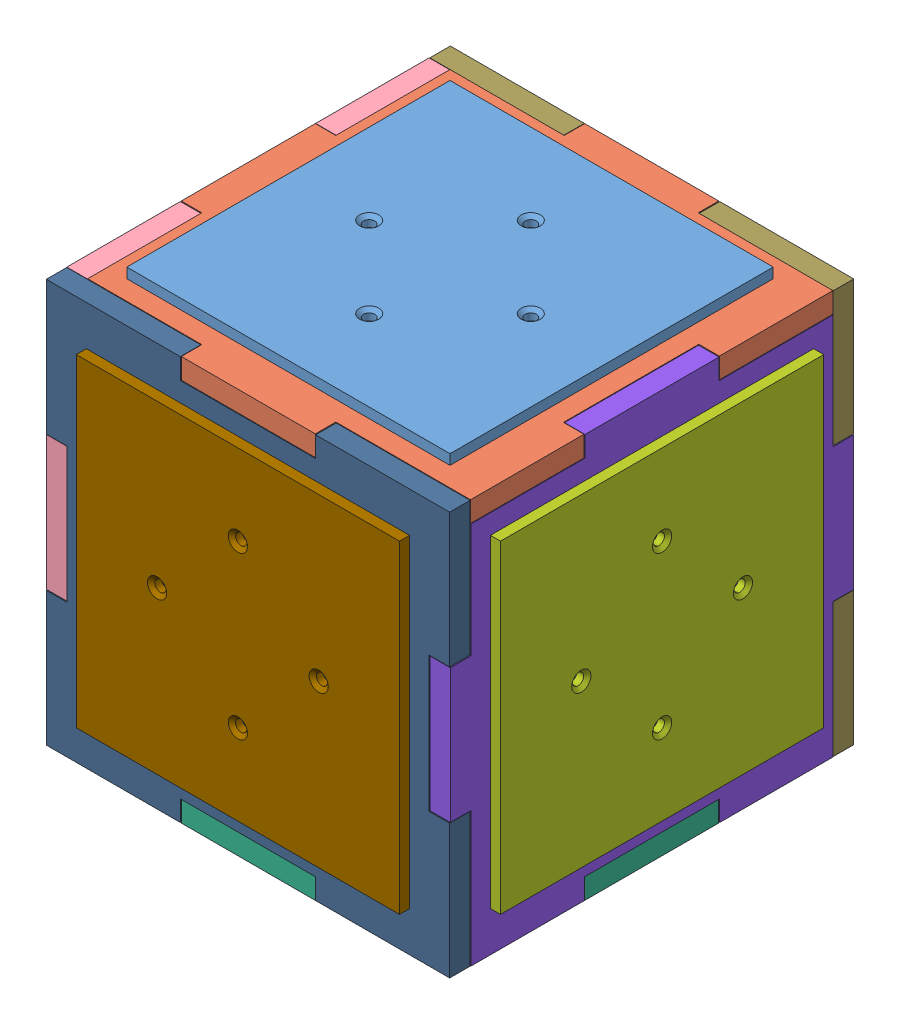
SolidWorks assembly cube_09, configuration cube09. Lengths in mm.
Overall size (66.67 66.67 66.67).
12 component instances, 12 part files, 6 mates.
Components (placement in the parent):
- panel_R^cube_09-13: panel_R^cube_09 [cube01] x (-1 0 0) z (0 0 1) size (50.8 1.59 50.8) (virtual)
- acrylic_R^cube_09-1: acrylic_R^cube_09 [A] at origin size (63.4 3.23 60.17) (virtual)
- panel_O^cube_09-8: panel_O^cube_09 [cube01] x (0 -1 0) z (0 0 1) size (50.8 1.59 54.98) (virtual)
- acrylic_O^cube_09-23: acrylic_O^cube_09 [A] x (0 1 0) z (0 0 1) size (63.4 3.23 60.17) (virtual)
- panel_Y^cube_09-9: panel_Y^cube_09 [cube01] at origin size (50.8 1.59 50.8) (virtual)
- acrylic_Y^cube_09-24: acrylic_Y^cube_09 [A] x (-1 0 0) z (0 0 1) size (63.4 3.23 63.4) (virtual)
- panel_G^cube_09-10: panel_G^cube_09 [cube01] x (0 1 0) z (0 0 1) size (50.8 1.59 50.8) (virtual)
- acrylic_G^cube_09-25: acrylic_G^cube_09 [A] x (0 -1 0) z (0 0 1) size (63.4 3.23 63.4) (virtual)
- panel_C^cube_09-11: panel_C^cube_09 [cube01] x (-1 0 0) z (0 -1 0) size (50.8 1.59 50.8) (virtual)
- acrylic_C^cube_09-26: acrylic_C^cube_09 [B] x (1 0 0) z (0 -1 0) size (63.4 3.23 63.4) (virtual)
- panel_B^cube_09-13: panel_B^cube_09 [cube01] x (-1 0 0) z (0 1 0) size (50.8 1.59 50.8) (virtual)
- acrylic_B^cube_09-27: acrylic_B^cube_09 [B] x (1 0 0) z (0 1 0) size (63.4 3.23 63.4) (virtual)
Mates (geometry in assembly coordinates):
- Coincident1: coincident aligned: plane of panel_R^cube_09-13 through (0 0 0) normal (0 0 1); plane of assembly through (0 0 0) normal (0 0 1)
- Coincident2: coincident anti-aligned: plane of panel_R^cube_09-13; plane of assembly through (0 0 0) normal (1 0 0)
- Coincident3: coincident anti-aligned: plane of panel_R^cube_09-13; plane of assembly through (0 0 0) normal (0 1 0)
- Coincident4: coincident aligned: plane of acrylic_R^cube_09-1 through (0 0 0) normal (0 0 1); plane of assembly through (0 0 0) normal (0 0 1)
- Coincident5: coincident aligned: plane of acrylic_R^cube_09-1 through (0 0 0) normal (1 0 0); plane of assembly through (0 0 0) normal (1 0 0)
- Coincident6: coincident aligned: plane of ? through (0 0 0) normal (0 1 0); plane of assembly through (0 0 0) normal (0 1 0)
